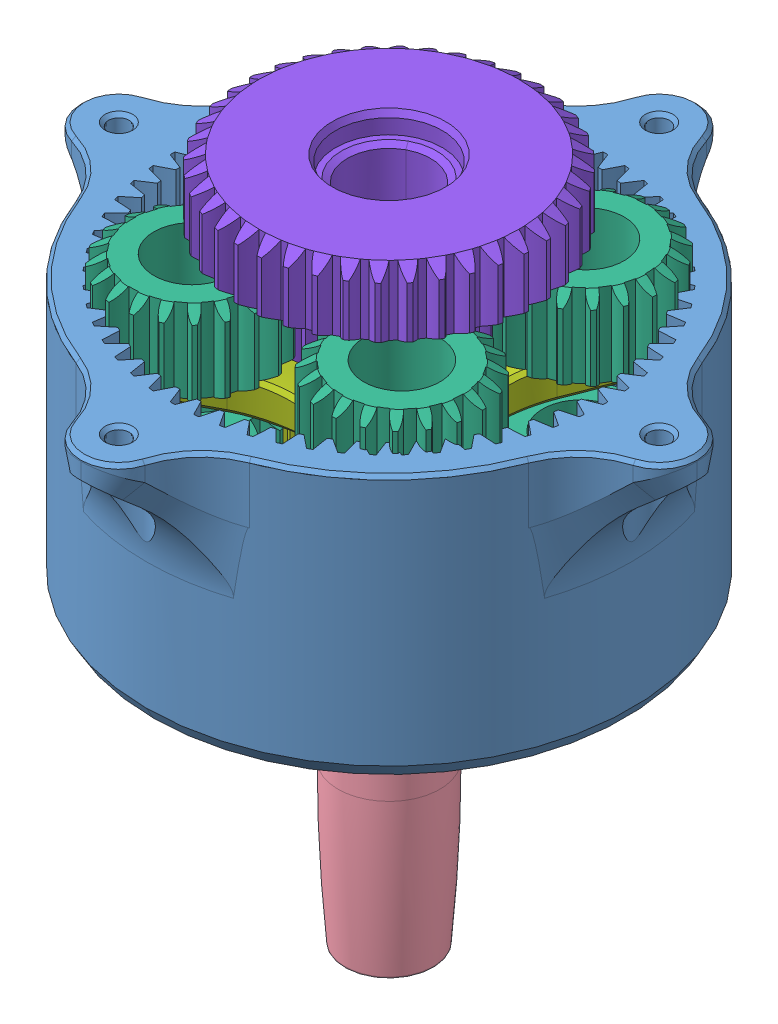
SolidWorks assembly 1.0. Altitude Gearbox Mk 1, configuration Default. Lengths in mm.
Overall size (89 98.98 89).
33 component instances, 8 part files, 46 mates.
Components (placement in the parent):
- Cap - Internal spur gear 1M 60T 18FW.step-1: Cap - Internal spur gear 1M 60T 18FW.step [Default] at (0 18 0) x (0 -1 0) z (0 0 1) size (38 89 89)
- 5909K13_Needle-Roller Thrust Bearing-1: 5909K13_Needle-Roller Thrust Bearing [5909K13] at (0 3 0) x (0.963316 0 -0.268371) z (0.268371 0 0.963316) size (28 2 28)
- Needle Roller Bearing - Washer-1: Needle Roller Bearing - Washer [Default] at (0 1 0) x (0.914016 0 -0.405677) z (0.405677 0 0.914016) size (28 1 28)
- Needle Roller Bearing - Washer-2: Needle Roller Bearing - Washer [Default] at (0 4 0) x (0.636199 0 -0.771525) z (0.771525 0 0.636199) size (28 1 28)
- Altitude Carrier Output-1: Altitude Carrier Output [Default] at (0 4 0) x (0.844222 0 -0.535993) z (0.535993 0 0.844222) size (50 59.48 50)
- M1 20T Bearing SubAssem-1: M1 20T Bearing SubAssem [Default] at (16.9267 12 -10.7467) x (0.874023 0 0.485885) z (0 -1 0) size (21.61 21.61 12)
  - 4668K252_Permanently Lubricated Stainless Steel Ball Bearing-1: 4668K252_Permanently Lubricated Stainless Steel Ball Bearing [4668K252] x (0.309017 -0.951057 0) z (0 0 1) size (15 15 4)
  - Metric - Spur gear 1M 20T back panel-1: Metric - Spur gear 1M 20T back panel [Default] at (0 0 2) x (0 0 -1) z (1 0 0) size (12 21.61 21.61)
- M1 20T Bearing SubAssem-2: M1 20T Bearing SubAssem [Default] at (-10.7467 12 -16.9267) x (0.497679 0 0.867361) z (0 -1 0) size (21.61 21.61 12)
  - 4668K252_Permanently Lubricated Stainless Steel Ball Bearing-1: 4668K252_Permanently Lubricated Stainless Steel Ball Bearing [4668K252] x (0.309017 -0.951057 0) z (0 0 1) size (15 15 4)
  - Metric - Spur gear 1M 20T back panel-1: Metric - Spur gear 1M 20T back panel [Default] at (0 0 2) x (0 0 -1) z (1 0 0) size (12 21.61 21.61)
- M1 20T Bearing SubAssem-3: M1 20T Bearing SubAssem [Default] at (-16.9267 12 10.7467) x (0.276887 0 0.960902) z (0 -1 0) size (21.61 21.61 12)
  - 4668K252_Permanently Lubricated Stainless Steel Ball Bearing-1: 4668K252_Permanently Lubricated Stainless Steel Ball Bearing [4668K252] x (0.309017 -0.951057 0) z (0 0 1) size (15 15 4)
  - Metric - Spur gear 1M 20T back panel-1: Metric - Spur gear 1M 20T back panel [Default] at (0 0 2) x (0 0 -1) z (1 0 0) size (12 21.61 21.61)
- M1 20T Bearing SubAssem-4: M1 20T Bearing SubAssem [Default] at (10.7467 12 16.9267) x (-0.256653 0 -0.966504) z (0 -1 0) size (21.61 21.61 12)
  - 4668K252_Permanently Lubricated Stainless Steel Ball Bearing-1: 4668K252_Permanently Lubricated Stainless Steel Ball Bearing [4668K252] x (0.309017 -0.951057 0) z (0 0 1) size (15 15 4)
  - Metric - Spur gear 1M 20T back panel-1: Metric - Spur gear 1M 20T back panel [Default] at (0 0 2) x (0 0 -1) z (1 0 0) size (12 21.61 21.61)
- altitude carrier and sun middle long-1: altitude carrier and sun middle long [Default] at (0 10 0) x (-0.659483 0 0.751719) z (-0.751719 0 -0.659483) size (50 24 50)
- M1 20T Bearing SubAssem-5: M1 20T Bearing SubAssem [Default] at (-15.1471 32 -13.2886) x (-0.387832 0 0.92173) z (0 -1 0) size (21.61 21.61 12)
  - 4668K252_Permanently Lubricated Stainless Steel Ball Bearing-1: 4668K252_Permanently Lubricated Stainless Steel Ball Bearing [4668K252] x (0.309017 -0.951057 0) z (0 0 1) size (15 15 4)
  - Metric - Spur gear 1M 20T back panel-1: Metric - Spur gear 1M 20T back panel [Default] at (0 0 2) x (0 0 -1) z (1 0 0) size (12 21.61 21.61)
- M1 20T Bearing SubAssem-6: M1 20T Bearing SubAssem [Default] at (-13.2886 32 15.1471) x (-0.794506 0 0.607256) z (0 -1 0) size (21.61 21.61 12)
  - 4668K252_Permanently Lubricated Stainless Steel Ball Bearing-1: 4668K252_Permanently Lubricated Stainless Steel Ball Bearing [4668K252] x (0.309017 -0.951057 0) z (0 0 1) size (15 15 4)
  - Metric - Spur gear 1M 20T back panel-1: Metric - Spur gear 1M 20T back panel [Default] at (0 0 2) x (0 0 -1) z (1 0 0) size (12 21.61 21.61)
- M1 20T Bearing SubAssem-7: M1 20T Bearing SubAssem [Default] at (13.2886 32 -15.1471) x (-0.240927 0 0.970543) z (0 -1 0) size (21.61 21.61 12)
  - 4668K252_Permanently Lubricated Stainless Steel Ball Bearing-1: 4668K252_Permanently Lubricated Stainless Steel Ball Bearing [4668K252] x (0.309017 -0.951057 0) z (0 0 1) size (15 15 4)
  - Metric - Spur gear 1M 20T back panel-1: Metric - Spur gear 1M 20T back panel [Default] at (0 0 2) x (0 0 -1) z (1 0 0) size (12 21.61 21.61)
- M1 20T Bearing SubAssem-8: M1 20T Bearing SubAssem [Default] at (15.1471 32 13.2886) x (-0.772007 0 -0.635614) z (0 -1 0) size (21.61 21.61 12)
  - 4668K252_Permanently Lubricated Stainless Steel Ball Bearing-1: 4668K252_Permanently Lubricated Stainless Steel Ball Bearing [4668K252] x (0.309017 -0.951057 0) z (0 0 1) size (15 15 4)
  - Metric - Spur gear 1M 20T back panel-1: Metric - Spur gear 1M 20T back panel [Default] at (0 0 2) x (0 0 -1) z (1 0 0) size (12 21.61 21.61)
- 4668K252_Permanently Lubricated Stainless Steel Ball Bearing-1: 4668K252_Permanently Lubricated Stainless Steel Ball Bearing [4668K252] at (0 12 0) x (1 0 0) z (0 -1 0) size (15 15 4)
- Altitude Input mk2-1: Altitude Input mk2 [Default] at (0 43.5 0) x (0 1 0) z (-0.475448 0 -0.879744) size (24 41.91 41.91)
- 4668K252_Permanently Lubricated Stainless Steel Ball Bearing-2: 4668K252_Permanently Lubricated Stainless Steel Ball Bearing [4668K252] at (0 31.5 0) x (0 0 1) z (0 -1 0) size (15 15 4)
Mates (geometry in assembly coordinates):
- Coincident1: coincident anti-aligned: plane of Cap - Internal spur gear 1M 60T 18FW.step-1 through (0 0 -29) normal (0 -1 0)
- Coincident2: coincident: point of Cap - Internal spur gear 1M 60T 18FW.step-1
- Coincident3: coincident: unknown of Cap - Internal spur gear 1M 60T 18FW.step-1
- Coincident4: coincident: unknown of Cap - Internal spur gear 1M 60T 18FW.step-1
- Concentric1: concentric anti-aligned: cylinder of Cap - Internal spur gear 1M 60T 18FW.step-1 through (0 1 0) axis (0 1 0) radius 14.15; cylinder of Needle Roller Bearing - Washer-1 through (0 2 0) axis (0 -1 0) radius 14
- Coincident5: coincident anti-aligned: plane of Cap - Internal spur gear 1M 60T 18FW.step-1 through (0 1 0) normal (0 1 0); plane of Needle Roller Bearing - Washer-1 through (0 1 0) normal (0 -1 0)
- Concentric2: concentric anti-aligned: cylinder of 5909K13_Needle-Roller Thrust Bearing-1 through (0 4 0) axis (0 1 0) radius 7.516; cone of Needle Roller Bearing - Washer-1 through (0 1.75 0) axis (0 -1 0)
- Tangent1: tangent anti-aligned: cylinder of 5909K13_Needle-Roller Thrust Bearing-1 through (-5.7183 3 -11.9525) axis (-0.431572 0 -0.902079) radius 1; plane of Needle Roller Bearing - Washer-1 through (0 2 0) normal (0 1 0)
- Concentric3: concentric anti-aligned: cylinder of 5909K13_Needle-Roller Thrust Bearing-1 through (0 4 0) axis (0 1 0) radius 7.516; circle of Needle Roller Bearing - Washer-2
- Tangent3: tangent anti-aligned: cylinder of 5909K13_Needle-Roller Thrust Bearing-1 through (-1.2855 3 -13.1875) axis (-0.097016 0 -0.995283) radius 1; plane of Needle Roller Bearing - Washer-2 through (0 4 0) normal (0 -1 0)
- Concentric4: concentric aligned: cylinder of 5909K13_Needle-Roller Thrust Bearing-1 through (0 4 0) axis (0 1 0) radius 7.516; cylinder of Altitude Carrier Output-1 through (0 -45 0) axis (0 1 0) radius 7.35
- Coincident6: coincident anti-aligned: plane of Needle Roller Bearing - Washer-2 through (0 5 0) normal (0 1 0); plane of Altitude Carrier Output-1 through (0 5 0) normal (0 -1 0)
- Concentric5: concentric aligned: cylinder of Altitude Carrier Output-1 through (16.9267 14 -10.7467) axis (0 -1 0) radius 4.95; cylinder of M1 20T Bearing SubAssem-1/4668K252_Permanently Lubricated Stainless Steel Ball Bearing-1 through (16.9267 10 -10.7467) axis (0 -1 0) radius 5
- Coincident7: coincident anti-aligned: plane of Altitude Carrier Output-1 through (0 10 0) normal (0 1 0); plane of M1 20T Bearing SubAssem-1/4668K252_Permanently Lubricated Stainless Steel Ball Bearing-1 through (20.4513 10 -6.9576) normal (0 -1 0)
- Concentric6: concentric aligned: cylinder of Altitude Carrier Output-1 through (-10.7467 14 -16.9267) axis (0 -1 0) radius 4.95; cylinder of M1 20T Bearing SubAssem-2/4668K252_Permanently Lubricated Stainless Steel Ball Bearing-1 through (-10.7467 10 -16.9267) axis (0 -1 0) radius 5
- Coincident8: coincident anti-aligned: plane of Altitude Carrier Output-1 through (0 10 0) normal (0 1 0); plane of M1 20T Bearing SubAssem-2/4668K252_Permanently Lubricated Stainless Steel Ball Bearing-1 through (-9.6843 10 -11.8619) normal (0 -1 0)
- Concentric7: concentric aligned: cylinder of Altitude Carrier Output-1 through (-16.9267 14 10.7467) axis (0 -1 0) radius 4.95; cylinder of M1 20T Bearing SubAssem-3/4668K252_Permanently Lubricated Stainless Steel Ball Bearing-1 through (-16.9267 10 10.7467) axis (0 -1 0) radius 5
- Coincident9: coincident anti-aligned: plane of Altitude Carrier Output-1 through (0 10 0) normal (0 1 0); plane of M1 20T Bearing SubAssem-3/4668K252_Permanently Lubricated Stainless Steel Ball Bearing-1 through (-17.1005 10 15.9187) normal (0 -1 0)
- Concentric8: concentric aligned: cylinder of Altitude Carrier Output-1 through (10.7467 14 16.9267) axis (0 -1 0) radius 4.95; cylinder of M1 20T Bearing SubAssem-4/4668K252_Permanently Lubricated Stainless Steel Ball Bearing-1 through (10.7467 10 16.9267) axis (0 -1 0) radius 5
- Coincident10: coincident anti-aligned: plane of Altitude Carrier Output-1 through (0 10 0) normal (0 1 0); plane of M1 20T Bearing SubAssem-4/4668K252_Permanently Lubricated Stainless Steel Ball Bearing-1 through (11.0291 10 11.7594) normal (0 -1 0)
- GearMate1: gear = 17.298 : 62.502 mm: cylinder of Cap - Internal spur gear 1M 60T 18FW.step-1 through (0 0 0) axis (0 1 0) radius 31.251; cylinder of M1 20T Bearing SubAssem-3/Metric - Spur gear 1M 20T back panel-1 through (-16.9267 10 10.7467) axis (0 1 0) radius 8.649
- GearMate2: gear = 62.502 : 17.298 mm: cylinder of M1 20T Bearing SubAssem-2/Metric - Spur gear 1M 20T back panel-1 through (-10.7467 10 -16.9267) axis (0 1 0) radius 8.649; cylinder of Cap - Internal spur gear 1M 60T 18FW.step-1 through (0 0 0) axis (0 1 0) radius 31.251
- GearMate4: gear = 62.502 : 17.298 mm: cylinder of M1 20T Bearing SubAssem-1/Metric - Spur gear 1M 20T back panel-1 through (16.9267 10 -10.7467) axis (0 1 0) radius 8.649; cylinder of Cap - Internal spur gear 1M 60T 18FW.step-1 through (0 0 0) axis (0 1 0) radius 31.251
- GearMate5: gear = 62.502 : 17.298 mm: cylinder of M1 20T Bearing SubAssem-4/Metric - Spur gear 1M 20T back panel-1 through (10.7467 10 16.9267) axis (0 1 0) radius 8.649; cylinder of Cap - Internal spur gear 1M 60T 18FW.step-1 through (0 0 0) axis (0 1 0) radius 31.251
- Concentric10: concentric anti-aligned: cylinder of altitude carrier and sun middle long-1 through (0 -12.6274 0) axis (0 1 0) radius 7.65; cylinder of 4668K252_Permanently Lubricated Stainless Steel Ball Bearing-1 through (0 10 0) axis (0 -1 0) radius 5
- Coincident11: coincident anti-aligned: plane of altitude carrier and sun middle long-1 through (0 14 0) normal (0 -1 0); plane of 4668K252_Permanently Lubricated Stainless Steel Ball Bearing-1 through (0 14 7.3845) normal (0 1 0)
- Concentric11: concentric aligned: cylinder of Cap - Internal spur gear 1M 60T 18FW.step-1 through (0 0 0) axis (0 1 0) radius 7.65; cylinder of altitude carrier and sun middle long-1 through (0 23.999 0) axis (0 1 0) radius 5.25
- Coincident12: coincident anti-aligned: plane of Altitude Carrier Output-1 through (0 10 0) normal (0 1 0); plane of 4668K252_Permanently Lubricated Stainless Steel Ball Bearing-1 through (0 10 5.175) normal (0 -1 0)
- GearMate6: gear = 17.298 : 17.498 mm: cylinder of altitude carrier and sun middle long-1 through (0 14 0) axis (0 -1 0) radius 8.749; cylinder of M1 20T Bearing SubAssem-4/Metric - Spur gear 1M 20T back panel-1 through (10.7467 10 16.9267) axis (0 1 0) radius 8.649
- Concentric13: concentric aligned: cylinder of altitude carrier and sun middle long-1 through (-15.1471 34 -13.2886) axis (0 -1 0) radius 4.85; cylinder of M1 20T Bearing SubAssem-5/4668K252_Permanently Lubricated Stainless Steel Ball Bearing-1 through (-15.1471 30 -13.2886) axis (0 -1 0) radius 5
- Concentric14: concentric aligned: cylinder of altitude carrier and sun middle long-1 through (13.2886 34 -15.1471) axis (0 -1 0) radius 4.85; cylinder of M1 20T Bearing SubAssem-7/4668K252_Permanently Lubricated Stainless Steel Ball Bearing-1 through (13.2886 30 -15.1471) axis (0 -1 0) radius 5
- Concentric15: concentric aligned: cylinder of altitude carrier and sun middle long-1 through (-13.2886 34 15.1471) axis (0 -1 0) radius 4.85; cylinder of M1 20T Bearing SubAssem-6/4668K252_Permanently Lubricated Stainless Steel Ball Bearing-1 through (-13.2886 30 15.1471) axis (0 -1 0) radius 5
- Concentric16: concentric aligned: cylinder of altitude carrier and sun middle long-1 through (15.1471 34 13.2886) axis (0 -1 0) radius 4.85; cylinder of M1 20T Bearing SubAssem-8/4668K252_Permanently Lubricated Stainless Steel Ball Bearing-1 through (15.1471 30 13.2886) axis (0 -1 0) radius 5
- Coincident13: coincident anti-aligned: plane of altitude carrier and sun middle long-1 through (0 30 0) normal (0 1 0); plane of M1 20T Bearing SubAssem-8/4668K252_Permanently Lubricated Stainless Steel Ball Bearing-1 through (12.364 30 8.9257) normal (0 -1 0)
- Coincident14: coincident anti-aligned: plane of altitude carrier and sun middle long-1 through (0 30 0) normal (0 1 0); plane of M1 20T Bearing SubAssem-6/4668K252_Permanently Lubricated Stainless Steel Ball Bearing-1 through (-18.17 30 16.8653) normal (0 -1 0)
- Coincident15: coincident anti-aligned: plane of altitude carrier and sun middle long-1 through (0 30 0) normal (0 1 0); plane of M1 20T Bearing SubAssem-5/4668K252_Permanently Lubricated Stainless Steel Ball Bearing-1 through (-18.5299 30 -9.3723) normal (0 -1 0)
- Coincident16: coincident anti-aligned: plane of altitude carrier and sun middle long-1 through (0 30 0) normal (0 1 0); plane of M1 20T Bearing SubAssem-7/4668K252_Permanently Lubricated Stainless Steel Ball Bearing-1 through (10.5508 30 -10.7557) normal (0 -1 0)
- GearMate7: gear = 62.502 : 17.298 mm: cylinder of M1 20T Bearing SubAssem-7/Metric - Spur gear 1M 20T back panel-1 through (13.2886 30 -15.1471) axis (0 1 0) radius 8.649; cylinder of Cap - Internal spur gear 1M 60T 18FW.step-1 through (0 0 0) axis (0 1 0) radius 31.251
- GearMate8: gear = 62.502 : 17.298 mm: cylinder of M1 20T Bearing SubAssem-5/Metric - Spur gear 1M 20T back panel-1 through (-15.1471 30 -13.2886) axis (0 1 0) radius 8.649; cylinder of Cap - Internal spur gear 1M 60T 18FW.step-1 through (0 0 0) axis (0 1 0) radius 31.251
- GearMate9: gear = 62.502 : 17.298 mm: cylinder of M1 20T Bearing SubAssem-6/Metric - Spur gear 1M 20T back panel-1 through (-13.2886 30 15.1471) axis (0 1 0) radius 8.649; cylinder of Cap - Internal spur gear 1M 60T 18FW.step-1 through (0 0 0) axis (0 1 0) radius 31.251
- GearMate10: gear = 17.298 : 62.502 mm: cylinder of Cap - Internal spur gear 1M 60T 18FW.step-1 through (0 0 0) axis (0 1 0) radius 31.251; cylinder of M1 20T Bearing SubAssem-8/Metric - Spur gear 1M 20T back panel-1 through (15.1471 30 13.2886) axis (0 1 0) radius 8.649
- Concentric18: concentric anti-aligned: cylinder of Altitude Input mk2-1 through (0 6.8726 0) axis (0 1 0) radius 7.65; cylinder of 4668K252_Permanently Lubricated Stainless Steel Ball Bearing-2 through (0 29.5 0) axis (0 -1 0) radius 7.5
- Coincident17: coincident aligned: plane of Altitude Input mk2-1 through (0 33.5 0) normal (0 -1 0); circle of 4668K252_Permanently Lubricated Stainless Steel Ball Bearing-2
- Concentric19: concentric aligned: cone of Needle Roller Bearing - Washer-1 through (0 1 0) axis (0 1 0); cylinder of Altitude Input mk2-1 through (0 33.5 0) axis (0 1 0) radius 5.25
- Distance1: distance = 1.5 mm anti-aligned: plane of M1 20T Bearing SubAssem-8/Metric - Spur gear 1M 20T back panel-1 through (10.9217 42 10.9267) normal (0 1 0); plane of Altitude Input mk2-1 through (0 43.5 0) normal (0 -1 0)
- GearMate11: gear = 17.298 : 17.498 mm: cylinder of Altitude Input mk2-1 through (0 33.5 0) axis (0 -1 0) radius 8.749; cylinder of M1 20T Bearing SubAssem-7/Metric - Spur gear 1M 20T back panel-1 through (13.2886 30 -15.1471) axis (0 1 0) radius 8.649
